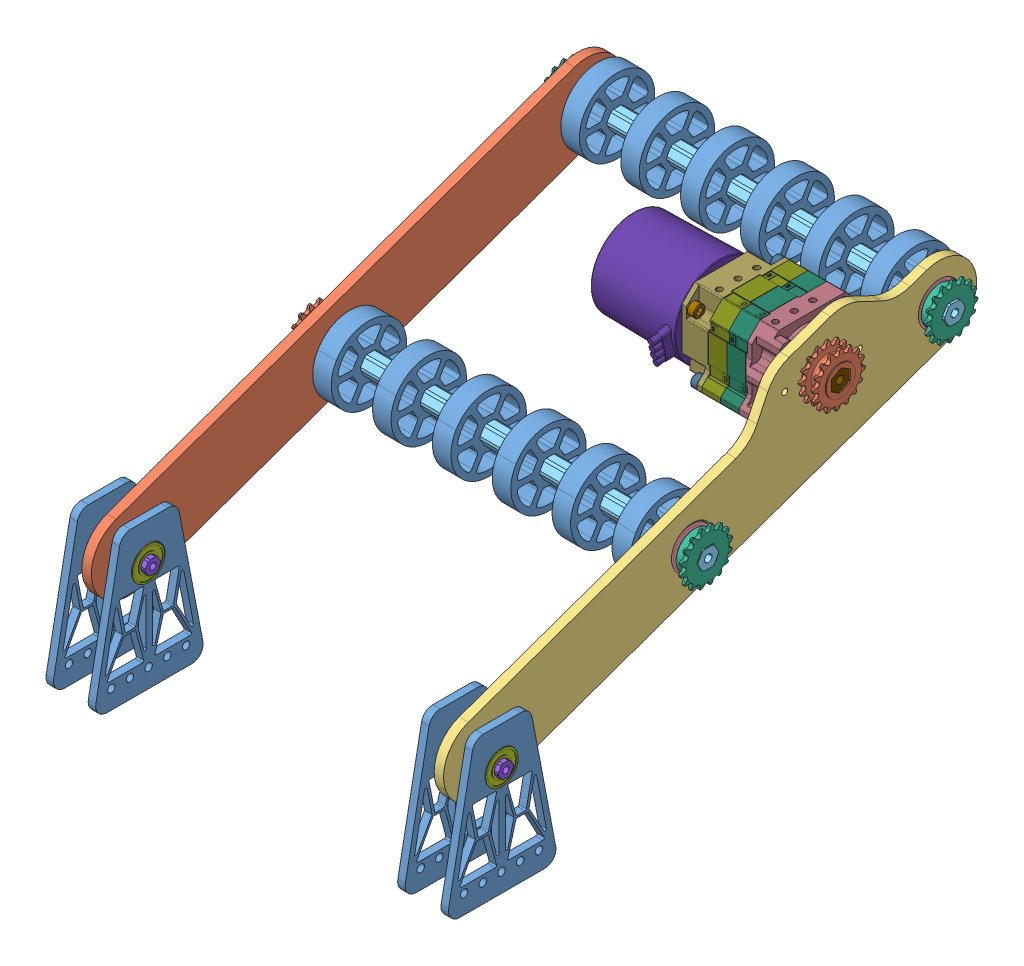
SolidWorks assembly arm intake, configuration Default. Lengths in mm.
Overall size (277.73 242.78 387.45).
54 component instances, 20 part files, 1 mates.
Components (placement in the parent):
- arm intake 1-1: arm intake 1 [Default] at (-43.4201 45.3163 126.9624) size (5.08 99.8 73.02)
- arm intake 1-2: arm intake 1 [Default] at (-14.6226 45.2934 127.1153) size (5.08 99.8 73.02)
- arm intake 2-1: arm intake 2 [Default] at (-28.4542 87.0656 105.9879) x (1 0 0) z (0 -0.333807 0.942641) size (6.35 50.8 381)
- arm intake 1-6: arm intake 1 [Default] at (225.3933 45.102 127.5601) size (5.08 99.8 73.02)
- arm intake 1-7: arm intake 1 [Default] at (195.948 45.0814 127.5601) size (5.08 99.8 73.02)
- arm intake 3-1: arm intake 3 [Default] at (210.8579 87.3995 106.1444) x (1 0 0) z (0 -0.333807 0.942641) size (6.35 77.74 381)
- 217-4006.step-7: 217-4006.step [Default] at (-24.2473 230.1789 -220.6767) x (0 0 -1) z (1 0 0) size (31.12 31.12 7.94)
- 217-4006.step-8: 217-4006.step [Default] at (212.5677 229.892 -220.5007) x (0 0 -1) z (-0.999962 -0.008727 0) size (31.12 31.12 7.94)
- 1_2thunderhex_10.5in-1: 1_2thunderhex_10.5in [Default] at (-229.3539 229.8833 -220.5211) x (0 0 -1) z (1 0 0) size (13.74 12.75 266.7)
- 16T_#25_500_hex_hubbed_sprocket_217-2642-1: 16T_#25_500_hex_hubbed_sprocket_217-2642 [Default] at (223.6465 229.5732 -220.5944) x (0 0.5 -0.866025) z (1 0 0) size (35.21 35.21 9.18)
- 16T_#25_500_hex_hubbed_sprocket_217-2642-2: 16T_#25_500_hex_hubbed_sprocket_217-2642 [Default] at (-34.9433 229.7883 -220.4698) x (0 -0.866025 0.5) z (-1 0 0) size (35.21 35.21 9.18)
- thunderhex_375_flanged_217-5829-1: thunderhex_375_flanged_217-5829 [Default] at (205.0802 119.409 90.1493) x (-0.999962 0 0.008727) z (-0.008727 0 -0.999962) size (7.11 24.61 24.61)
- thunderhex_375_flanged_217-5829-2: thunderhex_375_flanged_217-5829 [Default] at (209.1639 119.3357 90.1696) x (0.999962 0 -0.008727) z (0.008727 0 0.999962) size (7.11 24.61 24.61)
- thunderhex_375_flanged_217-5829-3: thunderhex_375_flanged_217-5829 [Default] at (223.6915 119.2761 90.0722) x (0.999962 0 -0.008727) z (0.008727 0 0.999962) size (7.11 24.61 24.61)
- 3_8thunderhex_1.5in-1: 3_8thunderhex_1.5in [Default] at (-223.6784 119.2112 90.035) x (0 0 -1) z (1 0 0) size (10.24 9.53 38.1)
- 3_8thunderhex_1.5in-2: 3_8thunderhex_1.5in [Default] at (-463.3119 119.2294 90.019) x (0 0 -1) z (1 0 0) size (10.24 9.53 38.1)
- thunderhex_375_flanged_217-5829-7: thunderhex_375_flanged_217-5829 [Default] at (-16.2694 119.2761 90.0722) x (0.999962 0 -0.008727) z (0.008727 0 0.999962) size (7.11 24.61 24.61)
- thunderhex_375_flanged_217-5829-8: thunderhex_375_flanged_217-5829 [Default] at (-30.1206 119.3357 90.1696) x (0.999962 0 -0.008727) z (0.008727 0 0.999962) size (7.11 24.61 24.61)
- thunderhex_375_flanged_217-5829-9: thunderhex_375_flanged_217-5829 [Default] at (-34.2043 119.409 90.1493) x (-0.999962 0 0.008727) z (-0.008727 0 -0.999962) size (7.11 24.61 24.61)
- MAXPlanetary 2-Stage-1: MAXPlanetary 2-Stage [Default] at (156.8829 230.5659 -141.0651) x (0 0 -1) z (1 0 0) size (89.61 89.51 122.08)
  - MAXPlanetary 2-Stage.STEP-1: MAXPlanetary 2-Stage.STEP [Default] at origin size (89.61 89.51 122.08)
    - REV-25-2109_2-Stage (No Shaft, For NEO).STEP-1: REV-25-2109_2-Stage (No Shaft, For NEO).STEP [Default] at origin size (65.15 54.03 73.34)
      - REV-25-2107_2-Stage.STEP-1: REV-25-2107_2-Stage.STEP [Default] at (0 0 6.35) x (-1 0 0) z (0 0 -1) size (65.15 54.03 73.34)
        - #10 Socket Head Cap Screws_0.500in Long.STEP-1: #10 Socket Head Cap Screws_0.500in Long.STEP [Default] at (21.1355 14.0872 12.7) x (0.923728 0.383049 0) z (0.383049 -0.923728 0) size (7.94 17.53 7.94)
        - #10 Socket Head Cap Screws_0.500in Long.STEP-2: #10 Socket Head Cap Screws_0.500in Long.STEP [Default] at (-21.1355 -14.0872 12.7) x (0.923728 0.383049 0) z (0.383049 -0.923728 0) size (7.94 17.53 7.94)
        - #10 Socket Head Cap Screws_1.500in Long.STEP-1: #10 Socket Head Cap Screws_1.500in Long.STEP [Default] at (-26.9919 21.4312 0) x (0.777574 0.628792 0) z (-0.628792 0.777574 0) size (7.94 42.93 7.94)
        - #10 Socket Head Cap Screws_1.500in Long.STEP-2: #10 Socket Head Cap Screws_1.500in Long.STEP [Default] at (26.9919 -21.4312 0) x (0.777574 0.628792 0) z (-0.628792 0.777574 0) size (7.94 42.93 7.94)
        - #10-32 Button Head Cap Screws_0.500in Long.STEP-1: #10-32 Button Head Cap Screws_0.500in Long.STEP [Default] at (0 0 -35.2425) x (0.655967 -0.754789 0) z (-0.754789 -0.655967 0) size (9.17 15.27 9.17)
      - REV-21-2106.STEP-1: REV-21-2106.STEP [Default] at origin size (61.91 50.8 19.05)
      - REV-21-2104.STEP-1: REV-21-2104.STEP [Default] at (0 0 44.45) x (0 0 1) z (-1 0 0) size (23.2 50.8 61.92)
      - REV-21-2108.STEP-1: REV-21-2108.STEP [Default] at (0 0 7.0985) x (-0.554615 -0.832107 0) z (0 0 -1) size (25.4 25.4 14.94)
    - REV-21-2101.STEP-1: REV-21-2101.STEP [Default] at (0 0 28.575) size (61.91 50.8 16.85)
    - REV-21-2102.STEP-1: REV-21-2102.STEP [Default] at (0 0 15.875) size (61.91 50.8 16.85)
    - REV-21-1650.STEP-1: REV-21-1650.STEP [Default] at (0 0 -9.525) x (0.554615 0.832107 0) z (0 0 1) size (64.41 64.76 93.26)
- 217-4006.step-9: 217-4006.step [Default] at (213.2861 230.5462 -141.2416) x (0 0 -1) z (-0.999962 -0.008727 0) size (31.12 31.12 7.94)
- 1_2thunderhex_1.5in-2: 1_2thunderhex_1.5in [Default] at (-228.1654 230.6457 -141.1828) x (0 0.999962 -0.008727) z (1 0 0) size (13.74 12.75 31.75)
- 16T_#25_500_hex_hubbed_sprocket_217-2642-3: 16T_#25_500_hex_hubbed_sprocket_217-2642 [Default] at (224.5937 169.5532 -53.1049) x (0 0.999657 -0.026177) z (1 0 0) size (35.21 35.21 9.18)
- WCP-0134.step-1: WCP-0134.step [Default] at (-7.812 231.1852 -220.5316) x (0.008727 0.507519 -0.861596) z (0.999962 -0.004429 0.007519) size (50.8 50.8 12.7)
- WCP-0134.step-2: WCP-0134.step [Default] at (32.828 231.1852 -220.5316) x (0.008727 0.507519 -0.861596) z (0.999962 -0.004429 0.007519) size (50.8 50.8 12.7)
- WCP-0134.step-3: WCP-0134.step [Default] at (73.468 231.1852 -220.5316) x (0.008727 0.507519 -0.861596) z (0.999962 -0.004429 0.007519) size (50.8 50.8 12.7)
- WCP-0134.step-4: WCP-0134.step [Default] at (114.108 231.1852 -220.5316) x (0.008727 0.507519 -0.861596) z (0.999962 -0.004429 0.007519) size (50.8 50.8 12.7)
- WCP-0134.step-5: WCP-0134.step [Default] at (154.748 231.1852 -220.5316) x (0.008727 0.507519 -0.861596) z (0.999962 -0.004429 0.007519) size (50.8 50.8 12.7)
- WCP-0134.step-6: WCP-0134.step [Default] at (195.388 231.1852 -220.5316) x (0.008727 0.507519 -0.861596) z (0.999962 -0.004429 0.007519) size (50.8 50.8 12.7)
- 217-4006.step-10: 217-4006.step [Default] at (212.6584 169.4978 -52.9854) x (0 0 -1) z (-0.999962 -0.008727 0) size (31.12 31.12 7.94)
- WCP-0134.step-7: WCP-0134.step [Default] at (195.4787 169.4664 -51.9368) x (0.008727 -0.507519 -0.861596) z (0.999962 0.004429 0.007519) size (50.8 50.8 12.7)
- WCP-0134.step-8: WCP-0134.step [Default] at (73.5587 169.4664 -51.9368) x (0.008727 -0.507519 -0.861596) z (0.999962 0.004429 0.007519) size (50.8 50.8 12.7)
- WCP-0134.step-9: WCP-0134.step [Default] at (154.8387 169.4664 -51.9368) x (0.008727 -0.507519 -0.861596) z (0.999962 0.004429 0.007519) size (50.8 50.8 12.7)
- WCP-0134.step-10: WCP-0134.step [Default] at (32.9187 169.4664 -51.9368) x (0.008727 -0.507519 -0.861596) z (0.999962 0.004429 0.007519) size (50.8 50.8 12.7)
- WCP-0134.step-11: WCP-0134.step [Default] at (114.1987 169.4664 -51.9368) x (0.008727 -0.507519 -0.861596) z (0.999962 0.004429 0.007519) size (50.8 50.8 12.7)
- WCP-0134.step-12: WCP-0134.step [Default] at (-7.7213 169.4664 -51.9368) x (0.008727 -0.507519 -0.861596) z (0.999962 0.004429 0.007519) size (50.8 50.8 12.7)
- 1_2thunderhex_10.5in-2: 1_2thunderhex_10.5in [Default] at (-229.2632 169.4892 -53.0058) x (0 0 -1) z (1 0 0) size (13.74 12.75 266.7)
- 217-4006.step-11: 217-4006.step [Default] at (-24.1566 169.7848 -53.1614) x (0 0 -1) z (1 0 0) size (31.12 31.12 7.94)
- WCP-0087.step-1: WCP-0087.step [Default] at (223.4657 230.6955 -141.2899) x (0 0.48481 -0.87462) z (1 0 0) size (35.45 35.45 12.45)
- WCP-0087.step-2: WCP-0087.step [Default] at (-34.7208 169.507 -52.8873) x (0 0 -1) z (1 0 0) size (35.45 35.45 12.45)
Mates (geometry in assembly coordinates):
- Coincident1: coincident anti-aligned: plane of arm intake 3-1 through (210.8579 87.3995 106.1444) normal (-1 0 0); plane of MAXPlanetary 2-Stage-1/MAXPlanetary 2-Stage.STEP-1/REV-25-2109_2-Stage (No Shaft, For NEO).STEP-1/REV-21-2104.STEP-1 through (210.8579 230.5659 -141.0651) normal (1 0 0)
